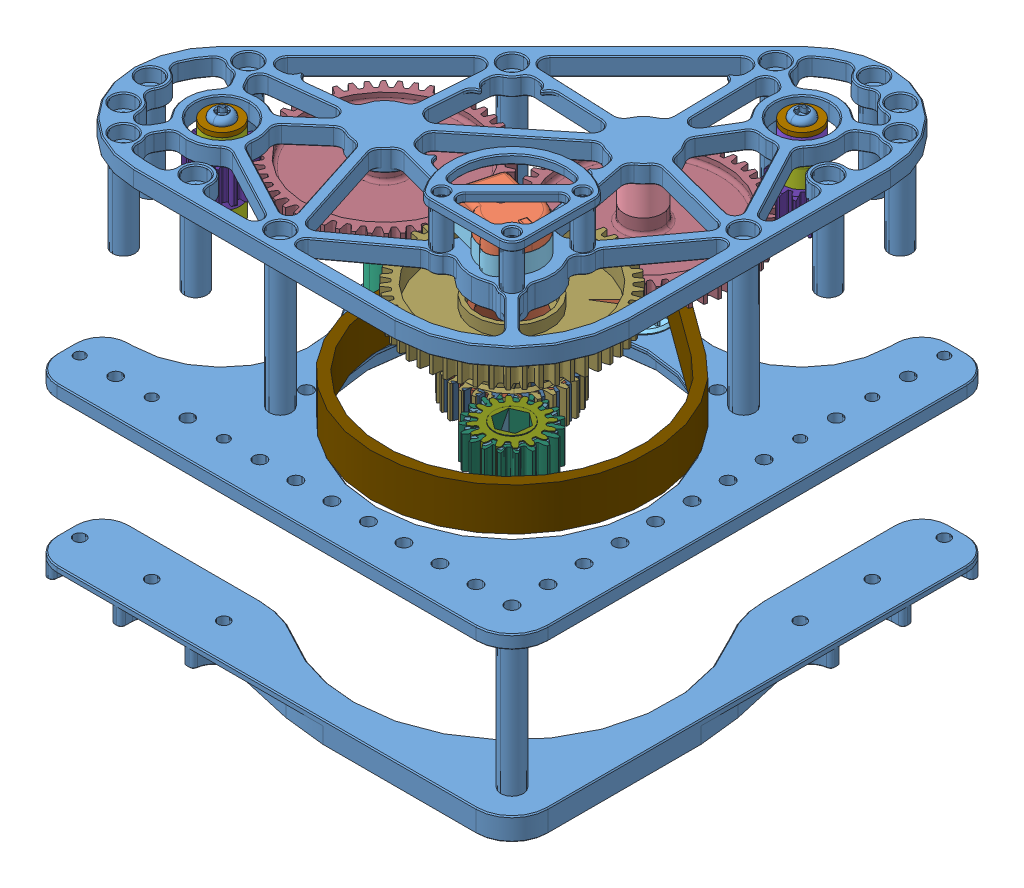
SolidWorks assembly MK4Frame, configuration Default. Lengths in mm.
Overall size (189.87 134.14 189.87).
34 component instances, 23 part files, 0 mates.
Components (placement in the parent):
- MK4i Master Part_Default Falcon 500 Config.STEP-1: MK4i Master Part_Default Falcon 500 Config.STEP [Default] at origin size (189.87 134.14 189.87)
- Bearing, R188ZZ, 217-3489.STEP-1: Bearing, R188ZZ, 217-3489.STEP [Default] at (-77.6314 97.6313 -123.9376) x (-0.188457 0 -0.982081) z (0.982081 0 -0.188457) size (12.7 4.76 12.7)
- Bearing, 688.STEP-1: Bearing, 688.STEP [Default] at (-77.6314 150.1375 -123.9376) x (0 -1 0) z (-0.336154 0 0.941807) size (5 16 16)
- MK4i Steering Shaft Spacer.STEP-1: MK4i Steering Shaft Spacer.STEP [Default] at (-77.6314 134.8105 -123.9376) x (-0.728275 0 -0.685285) z (0.685285 0 -0.728275) size (13.36 12.7 13.36)
- MK4i Steering Shaft Tall.STEP-1: MK4i Steering Shaft Tall.STEP [Default] at (-77.6314 152.5105 -123.9376) x (0.998641 0 -0.05212) z (0.05212 0 0.998641) size (17.78 57.04 17.78)
- MK4i Shaft, Drive Idler.STEP-1: MK4i Shaft, Drive Idler.STEP [Default] at (-128.0498 100.0125 -83.2602) size (13.36 56.18 13.36)
- Falcon Spacer .25.STEP-1: Falcon Spacer .25.STEP [Default] at (-158.75 123.7 -56.515) x (0.995401 0 0.095792) z (-0.095792 0 0.995401) size (12.7 6.35 12.7)
- Falcon Spacer .25.STEP-2: Falcon Spacer .25.STEP [Default] at (-158.75 145.925 -56.515) x (0.92897 0 -0.370156) z (0.370156 0 0.92897) size (12.7 6.35 12.7)
- Falcon Spacer .125.STEP-1: Falcon Spacer .125.STEP [Default] at (-56.515 149.1 -158.75) x (0.944247 0 -0.329237) z (0.329237 0 0.944247) size (12.7 3.17 12.7)
- Falcon Spacer .125.STEP-2: Falcon Spacer .125.STEP [Default] at (-158.75 130.05 -56.515) x (0.865282 0 -0.501286) z (0.501286 0 0.865282) size (12.7 3.17 12.7)
- Falcon Spacer .0625.STEP-1: Falcon Spacer .0625.STEP [Default] at (-158.75 152.275 -56.515) size (12.7 1.59 12.7)
- Falcon Spacer .0625.STEP-2: Falcon Spacer .0625.STEP [Default] at (-56.515 152.275 -158.75) x (0.982082 0 -0.188455) z (0.188455 0 0.982082) size (12.7 1.59 12.7)
- Falcon Spacer .25.STEP-3: Falcon Spacer .25.STEP [Default] at (-56.515 136.4 -158.75) size (12.7 6.35 12.7)
- Falcon Spacer .25.STEP-4: Falcon Spacer .25.STEP [Default] at (-56.515 142.75 -158.75) x (0.982082 0 -0.188455) z (0.188455 0 0.982082) size (12.7 6.35 12.7)
- Copy of topgears-1: Copy of topgears [Default] at origin size (163.42 43.94 160.87)
  - Double Gear, 20DP, 27T, 50T.STEP-1: Double Gear, 20DP, 27T, 50T.STEP [Default] at (-66.675 110.1225 -66.675) x (-0.730582 0 -0.682825) z (0 1 0) size (65.97 66.04 34.49)
  - Double Gear, 20DP, 25T, 50T.STEP-1: Double Gear, 20DP, 25T, 50T.STEP [Default] at (-66.675 110.1225 -66.675) x (-0.730582 0 -0.682825) z (0 1 0) size (65.97 66.04 34.49)
  - Double Gear, 20DP, 28T, 50T.STEP-1: Double Gear, 20DP, 28T, 50T.STEP [Default] at (-66.675 110.1225 -66.675) x (-0.730582 0 -0.682825) z (0 1 0) size (65.97 66.04 34.49)
  - Gear, 50T, 20DP, .375Hex.STEP-1: Gear, 50T, 20DP, .375Hex.STEP [Default] at (-128.0498 139.8651 -83.2602) x (0.985885 0 -0.167422) z (0 1 0) size (65.97 66.04 12.65)
  - Gear, 50T, 20DP, .375Hex.STEP-2: Gear, 50T, 20DP, .375Hex.STEP [Default] at (-77.6314 128.4859 -123.9376) x (-0.963721 0 0.266911) z (0 1 0) size (65.97 66.04 12.65)
  - Gear, 17T, 20DP, .375Hex.STEP-1: Gear, 17T, 20DP, .375Hex.STEP [Default] at (-46.8646 115.8367 -46.8646) x (0 1 0) z (0.115868 0 -0.993265) size (12.6 23.99 24.09)
  - Gear, 19T, 20DP, .375Hex.STEP-1: Gear, 19T, 20DP, .375Hex.STEP [Default] at (-46.8646 115.8367 -46.8646) x (0.115868 0 -0.993265) z (0.993265 0 0.115868) size (26.55 12.6 26.64)
  - Gear, 20DP, 16T, .375Hex, 217-5451.STEP-1: Gear, 20DP, 16T, .375Hex, 217-5451.STEP [Default] at (-46.8646 115.8375 -46.8646) x (0.993265 0 0.115868) z (0 -1 0) size (22.6 22.6 12.6)
  - Gear, 20DP 14T, Falcon Spline, am-4147.STEP-1: Gear, 20DP 14T, Falcon Spline, am-4147.STEP [Default] at (-56.515 123.7 -158.75) x (0 1 0) z (-0.155924 0 -0.987769) size (12.71 19.97 20.32)
  - Gear, 20DP 14T, Falcon Spline, am-4147.STEP-2: Gear, 20DP 14T, Falcon Spline, am-4147.STEP [Default] at (-158.75 133.225 -56.515) x (0 1 0) z (-0.622557 0 -0.782574) size (12.71 19.97 20.32)
  - Belt, 320-5M-15.STEP-1: Belt, 320-5M-15.STEP [Default] at (-66.675 109.752 -66.675) x (0.982183 0 -0.187927) z (0.187927 0 0.982183) size (97.78 15 116.29)
- Bearing, 688.STEP-2: Bearing, 688.STEP [Default] at (-128.0498 97.5125 -83.2602) x (0 -1 0) z (-0.444562 0 0.895748) size (5 16 16)
- Screw, Falcon 500 Pinion_90939A124.STEP-1: Screw, Falcon 500 Pinion_90939A124.STEP [Default] at (-56.515 153.8625 -158.75) x (1 0 0) z (0 1 0) size (7.93 7.93 14.91)
- Screw, Falcon 500 Pinion_90939A124.STEP-2: Screw, Falcon 500 Pinion_90939A124.STEP [Default] at (-158.75 153.8625 -56.515) x (0.982082 0 -0.188455) z (0 1 0) size (7.93 7.93 14.91)
- CANcoder Assembly.STEP-1: CANcoder Assembly.STEP [Default] at (-66.675 132.3975 -66.675) x (-0.260871 0 0.965374) z (0 1 0) size (21.75 26.91 13.52)
  - CANcoder Top Housing.STEP-1: CANcoder Top Housing.STEP [Default] at origin size (21.53 26.79 8.94)
  - CANcoder PCA.STEP-1: CANcoder PCA.STEP [Default] at (0 0 22.3055) size (15.93 23.27 3.19)
  - CANcoder Screw.STEP-1: CANcoder Screw.STEP [Default] at origin size (4.24 4.24 12.65)
  - CANcoder Bottom Housing.STEP-1: CANcoder Bottom Housing.STEP [Default] at origin size (21.75 26.91 6.35)
